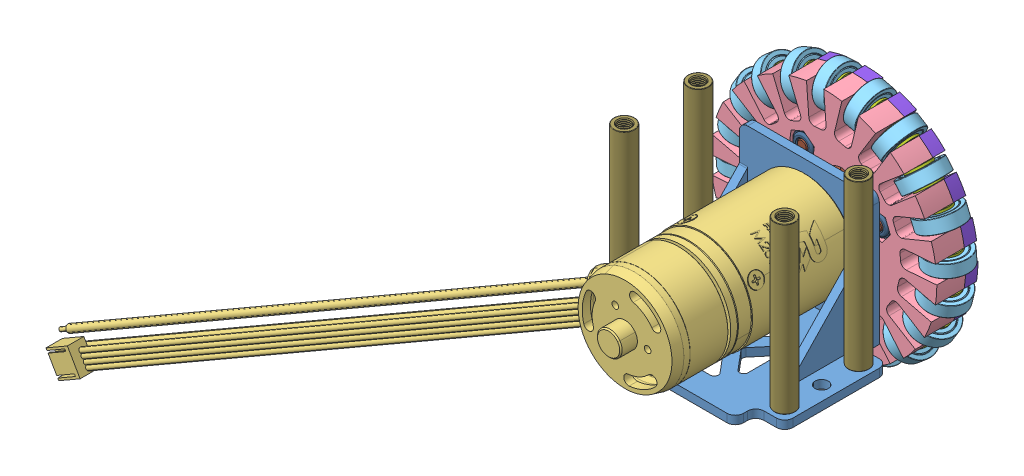
SolidWorks assembly RCSSL_gen2_OW_drive_unit, configuration Default. Lengths in mm.
Overall size (193.31 168.77 67.31).
123 component instances, 12 part files, 18 mates.
Components (placement in the parent):
- 1.5mm_aluminium_metal_plating_2006 motor mount-1: 1.5mm_aluminium_metal_plating_2006 motor mount [Default] at (10.7348 39.9667 23.6101) size (46 32 35)
- 3dp_AL_Gen2_Customised_AL_shaft_flange_connector_2006-1: 3dp_AL_Gen2_Customised_AL_shaft_flange_connector_2006 [Default] at (10.7348 39.9667 8.6101) x (0.866025 0.5 0) z (0 0 1) size (34 34 12.5)
- RoboMaster M2006 P36 motor 1-1: RoboMaster M2006 P36 motor 1 [默认] at (29.0021 49.1921 55.5053) x (0.258819 0.965926 0) z (0 0 1) size (137.53 138.78 64.81)
- ASM_RCssl_OW_Ver2-1: ASM_RCssl_OW_Ver2 [Default] at (25.0097 83.9716 -12.1645) x (-0.924615 -0.380903 0) z (0 0 1) size (59.33 59.33 15) (flexible)
  - 3dp_PETG_RCssl_OW_ver2_base-1: 3dp_PETG_RCssl_OW_ver2_base [Default] at (29.9603 35.2502 26.2746) size (54.84 54.84 7)
  - RCssl_OW_Ver2_roller_bearing_ASM-1: RCssl_OW_Ver2_roller_bearing_ASM [Default] at (24.4121 54.6156 21.3003) x (0 1 0) z (1 0 0) size (10 10 6)
    - BK_PU_68_3_10_3_bearing+roller-1: BK_PU_68_3_10_3_bearing+roller [Default] at (5.2981 6.4743 4.0482) size (10 10 3)
    - D3_H6_mid_axis-1: D3_H6_mid_axis [Default] at (5.2981 6.4743 2.5482) size (2.96 2.96 6)
    - m3_D6_H0.5_washer-1: m3_D6_H0.5_washer [Default] at (5.2981 6.4743 3.5482) x (0.872248 -0.489064 0) z (0 0 1) size (6 6 0.5)
    - m3_D6_H0.5_washer-2: m3_D6_H0.5_washer [Default] at (5.2981 6.4743 7.0482) size (6 6 0.5)
  - RCssl_OW_Ver2_roller_bearing_ASM-2: RCssl_OW_Ver2_roller_bearing_ASM [Default] at (30.6679 55.3823 21.3003) x (0.309017 0.951057 0) z (0.951057 -0.309017 0) size (10 10 6)
    - BK_PU_68_3_10_3_bearing+roller-1: BK_PU_68_3_10_3_bearing+roller [Default] at (5.2981 6.4743 4.0482) size (10 10 3)
    - D3_H6_mid_axis-1: D3_H6_mid_axis [Default] at (5.2981 6.4743 2.5482) size (2.96 2.96 6)
    - m3_D6_H0.5_washer-1: m3_D6_H0.5_washer [Default] at (5.2981 6.4743 3.5482) x (0.872248 -0.489064 0) z (0 0 1) size (6 6 0.5)
    - m3_D6_H0.5_washer-2: m3_D6_H0.5_washer [Default] at (5.2981 6.4743 7.0482) size (6 6 0.5)
  - RCssl_OW_Ver2_roller_bearing_ASM-3: RCssl_OW_Ver2_roller_bearing_ASM [Default] at (36.8544 54.1783 21.3003) x (0.587785 0.809017 0) z (0.809017 -0.587785 0) size (10 10 6)
    - BK_PU_68_3_10_3_bearing+roller-1: BK_PU_68_3_10_3_bearing+roller [Default] at (5.2981 6.4743 4.0482) size (10 10 3)
    - D3_H6_mid_axis-1: D3_H6_mid_axis [Default] at (5.2981 6.4743 2.5482) size (2.96 2.96 6)
    - m3_D6_H0.5_washer-1: m3_D6_H0.5_washer [Default] at (5.2981 6.4743 3.5482) x (0.872248 -0.489064 0) z (0 0 1) size (6 6 0.5)
    - m3_D6_H0.5_washer-2: m3_D6_H0.5_washer [Default] at (5.2981 6.4743 7.0482) size (6 6 0.5)
  - RCssl_OW_Ver2_roller_bearing_ASM-4: RCssl_OW_Ver2_roller_bearing_ASM [Default] at (42.3661 51.1215 21.3003) x (0.809017 0.587785 0) z (0.587785 -0.809017 0) size (10 10 6)
    - BK_PU_68_3_10_3_bearing+roller-1: BK_PU_68_3_10_3_bearing+roller [Default] at (5.2981 6.4743 4.0482) size (10 10 3)
    - D3_H6_mid_axis-1: D3_H6_mid_axis [Default] at (5.2981 6.4743 2.5482) size (2.96 2.96 6)
    - m3_D6_H0.5_washer-1: m3_D6_H0.5_washer [Default] at (5.2981 6.4743 3.5482) x (0.872248 -0.489064 0) z (0 0 1) size (6 6 0.5)
    - m3_D6_H0.5_washer-2: m3_D6_H0.5_washer [Default] at (5.2981 6.4743 7.0482) size (6 6 0.5)
  - RCssl_OW_Ver2_roller_bearing_ASM-5: RCssl_OW_Ver2_roller_bearing_ASM [Default] at (46.6634 46.5111 21.3003) x (0.951057 0.309017 0) z (0.309017 -0.951057 0) size (10 10 6)
    - BK_PU_68_3_10_3_bearing+roller-1: BK_PU_68_3_10_3_bearing+roller [Default] at (5.2981 6.4743 4.0482) size (10 10 3)
    - D3_H6_mid_axis-1: D3_H6_mid_axis [Default] at (5.2981 6.4743 2.5482) size (2.96 2.96 6)
    - m3_D6_H0.5_washer-1: m3_D6_H0.5_washer [Default] at (5.2981 6.4743 3.5482) x (0.872248 -0.489064 0) z (0 0 1) size (6 6 0.5)
    - m3_D6_H0.5_washer-2: m3_D6_H0.5_washer [Default] at (5.2981 6.4743 7.0482) size (6 6 0.5)
  - RCssl_OW_Ver2_roller_bearing_ASM-6: RCssl_OW_Ver2_roller_bearing_ASM [Default] at (49.3257 40.7985 21.3003) x (1 0 0) z (0 -1 0) size (10 10 6)
    - BK_PU_68_3_10_3_bearing+roller-1: BK_PU_68_3_10_3_bearing+roller [Default] at (5.2981 6.4743 4.0482) size (10 10 3)
    - D3_H6_mid_axis-1: D3_H6_mid_axis [Default] at (5.2981 6.4743 2.5482) size (2.96 2.96 6)
    - m3_D6_H0.5_washer-1: m3_D6_H0.5_washer [Default] at (5.2981 6.4743 3.5482) x (0.872248 -0.489064 0) z (0 0 1) size (6 6 0.5)
    - m3_D6_H0.5_washer-2: m3_D6_H0.5_washer [Default] at (5.2981 6.4743 7.0482) size (6 6 0.5)
  - RCssl_OW_Ver2_roller_bearing_ASM-7: RCssl_OW_Ver2_roller_bearing_ASM [Default] at (50.0924 34.5427 21.3003) x (0.951057 -0.309017 0) z (-0.309017 -0.951057 0) size (10 10 6)
    - BK_PU_68_3_10_3_bearing+roller-1: BK_PU_68_3_10_3_bearing+roller [Default] at (5.2981 6.4743 4.0482) size (10 10 3)
    - D3_H6_mid_axis-1: D3_H6_mid_axis [Default] at (5.2981 6.4743 2.5482) size (2.96 2.96 6)
    - m3_D6_H0.5_washer-1: m3_D6_H0.5_washer [Default] at (5.2981 6.4743 3.5482) x (0.872248 -0.489064 0) z (0 0 1) size (6 6 0.5)
    - m3_D6_H0.5_washer-2: m3_D6_H0.5_washer [Default] at (5.2981 6.4743 7.0482) size (6 6 0.5)
  - RCssl_OW_Ver2_roller_bearing_ASM-8: RCssl_OW_Ver2_roller_bearing_ASM [Default] at (48.8884 28.3562 21.3003) x (0.809017 -0.587785 0) z (-0.587785 -0.809017 0) size (10 10 6)
    - BK_PU_68_3_10_3_bearing+roller-1: BK_PU_68_3_10_3_bearing+roller [Default] at (5.2981 6.4743 4.0482) size (10 10 3)
    - D3_H6_mid_axis-1: D3_H6_mid_axis [Default] at (5.2981 6.4743 2.5482) size (2.96 2.96 6)
    - m3_D6_H0.5_washer-1: m3_D6_H0.5_washer [Default] at (5.2981 6.4743 3.5482) x (0.872248 -0.489064 0) z (0 0 1) size (6 6 0.5)
    - m3_D6_H0.5_washer-2: m3_D6_H0.5_washer [Default] at (5.2981 6.4743 7.0482) size (6 6 0.5)
  - RCssl_OW_Ver2_roller_bearing_ASM-9: RCssl_OW_Ver2_roller_bearing_ASM [Default] at (45.8316 22.8445 21.3003) x (0.587785 -0.809017 0) z (-0.809017 -0.587785 0) size (10 10 6)
    - BK_PU_68_3_10_3_bearing+roller-1: BK_PU_68_3_10_3_bearing+roller [Default] at (5.2981 6.4743 4.0482) size (10 10 3)
    - D3_H6_mid_axis-1: D3_H6_mid_axis [Default] at (5.2981 6.4743 2.5482) size (2.96 2.96 6)
    - m3_D6_H0.5_washer-1: m3_D6_H0.5_washer [Default] at (5.2981 6.4743 3.5482) x (0.872248 -0.489064 0) z (0 0 1) size (6 6 0.5)
    - m3_D6_H0.5_washer-2: m3_D6_H0.5_washer [Default] at (5.2981 6.4743 7.0482) size (6 6 0.5)
  - RCssl_OW_Ver2_roller_bearing_ASM-10: RCssl_OW_Ver2_roller_bearing_ASM [Default] at (41.2212 18.5472 21.3003) x (0.309017 -0.951057 0) z (-0.951057 -0.309017 0) size (10 10 6)
    - BK_PU_68_3_10_3_bearing+roller-1: BK_PU_68_3_10_3_bearing+roller [Default] at (5.2981 6.4743 4.0482) size (10 10 3)
    - D3_H6_mid_axis-1: D3_H6_mid_axis [Default] at (5.2981 6.4743 2.5482) size (2.96 2.96 6)
    - m3_D6_H0.5_washer-1: m3_D6_H0.5_washer [Default] at (5.2981 6.4743 3.5482) x (0.872248 -0.489064 0) z (0 0 1) size (6 6 0.5)
    - m3_D6_H0.5_washer-2: m3_D6_H0.5_washer [Default] at (5.2981 6.4743 7.0482) size (6 6 0.5)
  - RCssl_OW_Ver2_roller_bearing_ASM-11: RCssl_OW_Ver2_roller_bearing_ASM [Default] at (35.5086 15.8849 21.3003) x (0 -1 0) z (-1 0 0) size (10 10 6)
    - BK_PU_68_3_10_3_bearing+roller-1: BK_PU_68_3_10_3_bearing+roller [Default] at (5.2981 6.4743 4.0482) size (10 10 3)
    - D3_H6_mid_axis-1: D3_H6_mid_axis [Default] at (5.2981 6.4743 2.5482) size (2.96 2.96 6)
    - m3_D6_H0.5_washer-1: m3_D6_H0.5_washer [Default] at (5.2981 6.4743 3.5482) x (0.872248 -0.489064 0) z (0 0 1) size (6 6 0.5)
    - m3_D6_H0.5_washer-2: m3_D6_H0.5_washer [Default] at (5.2981 6.4743 7.0482) size (6 6 0.5)
  - RCssl_OW_Ver2_roller_bearing_ASM-12: RCssl_OW_Ver2_roller_bearing_ASM [Default] at (29.2528 15.1182 21.3003) x (-0.309017 -0.951057 0) z (-0.951057 0.309017 0) size (10 10 6)
    - BK_PU_68_3_10_3_bearing+roller-1: BK_PU_68_3_10_3_bearing+roller [Default] at (5.2981 6.4743 4.0482) size (10 10 3)
    - D3_H6_mid_axis-1: D3_H6_mid_axis [Default] at (5.2981 6.4743 2.5482) size (2.96 2.96 6)
    - m3_D6_H0.5_washer-1: m3_D6_H0.5_washer [Default] at (5.2981 6.4743 3.5482) x (0.872248 -0.489064 0) z (0 0 1) size (6 6 0.5)
    - m3_D6_H0.5_washer-2: m3_D6_H0.5_washer [Default] at (5.2981 6.4743 7.0482) size (6 6 0.5)
  - RCssl_OW_Ver2_roller_bearing_ASM-13: RCssl_OW_Ver2_roller_bearing_ASM [Default] at (23.0663 16.3222 21.3003) x (-0.587785 -0.809017 0) z (-0.809017 0.587785 0) size (10 10 6)
    - BK_PU_68_3_10_3_bearing+roller-1: BK_PU_68_3_10_3_bearing+roller [Default] at (5.2981 6.4743 4.0482) size (10 10 3)
    - D3_H6_mid_axis-1: D3_H6_mid_axis [Default] at (5.2981 6.4743 2.5482) size (2.96 2.96 6)
    - m3_D6_H0.5_washer-1: m3_D6_H0.5_washer [Default] at (5.2981 6.4743 3.5482) x (0.872248 -0.489064 0) z (0 0 1) size (6 6 0.5)
    - m3_D6_H0.5_washer-2: m3_D6_H0.5_washer [Default] at (5.2981 6.4743 7.0482) size (6 6 0.5)
  - RCssl_OW_Ver2_roller_bearing_ASM-14: RCssl_OW_Ver2_roller_bearing_ASM [Default] at (17.5546 19.379 21.3003) x (-0.809017 -0.587785 0) z (-0.587785 0.809017 0) size (10 10 6)
    - BK_PU_68_3_10_3_bearing+roller-1: BK_PU_68_3_10_3_bearing+roller [Default] at (5.2981 6.4743 4.0482) size (10 10 3)
    - D3_H6_mid_axis-1: D3_H6_mid_axis [Default] at (5.2981 6.4743 2.5482) size (2.96 2.96 6)
    - m3_D6_H0.5_washer-1: m3_D6_H0.5_washer [Default] at (5.2981 6.4743 3.5482) x (0.872248 -0.489064 0) z (0 0 1) size (6 6 0.5)
    - m3_D6_H0.5_washer-2: m3_D6_H0.5_washer [Default] at (5.2981 6.4743 7.0482) size (6 6 0.5)
  - RCssl_OW_Ver2_roller_bearing_ASM-15: RCssl_OW_Ver2_roller_bearing_ASM [Default] at (13.2573 23.9893 21.3003) x (-0.951057 -0.309017 0) z (-0.309017 0.951057 0) size (10 10 6)
    - BK_PU_68_3_10_3_bearing+roller-1: BK_PU_68_3_10_3_bearing+roller [Default] at (5.2981 6.4743 4.0482) size (10 10 3)
    - D3_H6_mid_axis-1: D3_H6_mid_axis [Default] at (5.2981 6.4743 2.5482) size (2.96 2.96 6)
    - m3_D6_H0.5_washer-1: m3_D6_H0.5_washer [Default] at (5.2981 6.4743 3.5482) x (0.872248 -0.489064 0) z (0 0 1) size (6 6 0.5)
    - m3_D6_H0.5_washer-2: m3_D6_H0.5_washer [Default] at (5.2981 6.4743 7.0482) size (6 6 0.5)
  - RCssl_OW_Ver2_roller_bearing_ASM-16: RCssl_OW_Ver2_roller_bearing_ASM [Default] at (10.595 29.702 21.3003) x (-1 0 0) z (0 1 0) size (10 10 6)
    - BK_PU_68_3_10_3_bearing+roller-1: BK_PU_68_3_10_3_bearing+roller [Default] at (5.2981 6.4743 4.0482) size (10 10 3)
    - D3_H6_mid_axis-1: D3_H6_mid_axis [Default] at (5.2981 6.4743 2.5482) size (2.96 2.96 6)
    - m3_D6_H0.5_washer-1: m3_D6_H0.5_washer [Default] at (5.2981 6.4743 3.5482) x (0.872248 -0.489064 0) z (0 0 1) size (6 6 0.5)
    - m3_D6_H0.5_washer-2: m3_D6_H0.5_washer [Default] at (5.2981 6.4743 7.0482) size (6 6 0.5)
  - RCssl_OW_Ver2_roller_bearing_ASM-17: RCssl_OW_Ver2_roller_bearing_ASM [Default] at (9.8283 35.9578 21.3003) x (-0.951057 0.309017 0) z (0.309017 0.951057 0) size (10 10 6)
    - BK_PU_68_3_10_3_bearing+roller-1: BK_PU_68_3_10_3_bearing+roller [Default] at (5.2981 6.4743 4.0482) size (10 10 3)
    - D3_H6_mid_axis-1: D3_H6_mid_axis [Default] at (5.2981 6.4743 2.5482) size (2.96 2.96 6)
    - m3_D6_H0.5_washer-1: m3_D6_H0.5_washer [Default] at (5.2981 6.4743 3.5482) x (0.872248 -0.489064 0) z (0 0 1) size (6 6 0.5)
    - m3_D6_H0.5_washer-2: m3_D6_H0.5_washer [Default] at (5.2981 6.4743 7.0482) size (6 6 0.5)
  - RCssl_OW_Ver2_roller_bearing_ASM-18: RCssl_OW_Ver2_roller_bearing_ASM [Default] at (11.0323 42.1443 21.3003) x (-0.809017 0.587785 0) z (0.587785 0.809017 0) size (10 10 6)
    - BK_PU_68_3_10_3_bearing+roller-1: BK_PU_68_3_10_3_bearing+roller [Default] at (5.2981 6.4743 4.0482) size (10 10 3)
    - D3_H6_mid_axis-1: D3_H6_mid_axis [Default] at (5.2981 6.4743 2.5482) size (2.96 2.96 6)
    - m3_D6_H0.5_washer-1: m3_D6_H0.5_washer [Default] at (5.2981 6.4743 3.5482) x (0.872248 -0.489064 0) z (0 0 1) size (6 6 0.5)
    - m3_D6_H0.5_washer-2: m3_D6_H0.5_washer [Default] at (5.2981 6.4743 7.0482) size (6 6 0.5)
  - RCssl_OW_Ver2_roller_bearing_ASM-19: RCssl_OW_Ver2_roller_bearing_ASM [Default] at (14.0891 47.656 21.3003) x (-0.587785 0.809017 0) z (0.809017 0.587785 0) size (10 10 6) (flexible)
    - BK_PU_68_3_10_3_bearing+roller-1: BK_PU_68_3_10_3_bearing+roller [Default] at (5.2981 6.4743 4.0482) size (10 10 3)
    - D3_H6_mid_axis-1: D3_H6_mid_axis [Default] at (5.2981 6.4743 2.5482) size (2.96 2.96 6)
    - m3_D6_H0.5_washer-1: m3_D6_H0.5_washer [Default] at (5.2981 6.4743 3.5482) x (0.872248 -0.489064 0) z (0 0 1) size (6 6 0.5)
    - m3_D6_H0.5_washer-2: m3_D6_H0.5_washer [Default] at (5.2981 6.4743 7.0482) size (6 6 0.5)
  - RCssl_OW_Ver2_roller_bearing_ASM-20: RCssl_OW_Ver2_roller_bearing_ASM [Default] at (18.6994 51.9533 21.3003) x (-0.309017 0.951057 0) z (0.951057 0.309017 0) size (10 10 6)
    - BK_PU_68_3_10_3_bearing+roller-1: BK_PU_68_3_10_3_bearing+roller [Default] at (5.2981 6.4743 4.0482) size (10 10 3)
    - D3_H6_mid_axis-1: D3_H6_mid_axis [Default] at (5.2981 6.4743 2.5482) size (2.96 2.96 6)
    - m3_D6_H0.5_washer-1: m3_D6_H0.5_washer [Default] at (5.2981 6.4743 3.5482) x (0.872248 -0.489064 0) z (0 0 1) size (6 6 0.5)
    - m3_D6_H0.5_washer-2: m3_D6_H0.5_washer [Default] at (5.2981 6.4743 7.0482) size (6 6 0.5)
  - CF3mm_OW_gen2_output_plane-1: CF3mm_OW_gen2_output_plane [Default] at (29.9603 35.2502 44.7746) size (54.84 54.84 3)
  - 3dp_PETG_RCssl_OW_front_lock-1: 3dp_PETG_RCssl_OW_front_lock [Default] at (29.9603 35.2502 21.2746) x (1 0 0) z (0 0 -1) size (21.15 21.15 4.13)
  - nut_din_985-m3x0_5-8-1: nut_din_985-m3x0_5-8 [Default] at (29.9603 21.2502 29.2746) x (-1 0 0) z (0 0 -1) size (6.2 5.5 4)
  - nut_din_985-m3x0_5-8-2: nut_din_985-m3x0_5-8 [Default] at (15.9603 35.2502 29.2746) x (0 1 0) z (0 0 -1) size (6.2 5.5 4)
  - nut_din_985-m3x0_5-8-3: nut_din_985-m3x0_5-8 [Default] at (29.9603 49.2502 29.2746) x (1 0 0) z (0 0 -1) size (6.2 5.5 4)
  - nut_din_985-m3x0_5-8-4: nut_din_985-m3x0_5-8 [Default] at (43.9603 35.2502 29.2746) x (0 -1 0) z (0 0 -1) size (6.2 5.5 4)
  - M3_304__full_teeth__screw_10mm-1: M3_304__full_teeth__screw_10mm [Default] at (29.992 49.2503 23.2746) x (-0.002323 0.999997 0) z (0 0 -1) size (5.3 5.3 13)
  - M3_304__full_teeth__screw_10mm-2: M3_304__full_teeth__screw_10mm [Default] at (43.9604 35.2186 23.2746) x (0.999997 0.002323 0) z (0 0 -1) size (5.3 5.3 13)
  - M3_304__full_teeth__screw_10mm-3: M3_304__full_teeth__screw_10mm [Default] at (29.9287 21.2502 23.2746) x (0.002323 -0.999997 0) z (0 0 -1) size (5.3 5.3 13)
  - M3_304__full_teeth__screw_10mm-4: M3_304__full_teeth__screw_10mm [Default] at (15.9603 35.2819 23.2746) x (-0.999997 -0.002323 0) z (0 0 -1) size (5.3 5.3 13)
  - M3_304__full_teeth__screw_10mm-5: M3_304__full_teeth__screw_10mm [Default] at (37.0442 42.2923 21.2746) x (0.914728 0.40407 0) z (0 0 -1) size (5.3 5.3 13)
  - M3_304__full_teeth__screw_10mm-6: M3_304__full_teeth__screw_10mm [Default] at (37.0024 28.1664 21.2746) x (0.40407 -0.914728 0) z (0 0 -1) size (5.3 5.3 13)
  - M3_304__full_teeth__screw_10mm-7: M3_304__full_teeth__screw_10mm [Default] at (22.8765 28.2081 21.2746) x (-0.914728 -0.40407 0) z (0 0 -1) size (5.3 5.3 13)
  - M3_304__full_teeth__screw_10mm-8: M3_304__full_teeth__screw_10mm [Default] at (22.9182 42.3341 21.2746) x (-0.40407 0.914728 0) z (0 0 -1) size (5.3 5.3 13)
- AL_pillar_M3_D6_H40_Threaded-2: AL_pillar_M3_D6_H40_Threaded [H30] at (-8.7652 24.9667 50.1101) size (5 40 5)
- AL_pillar_M3_D6_H40_Threaded-3: AL_pillar_M3_D6_H40_Threaded [H30] at (30.2348 24.9667 50.1101) size (5 40 5)
- AL_pillar_M3_D6_H40_Threaded-4: AL_pillar_M3_D6_H40_Threaded [Default] at (30.2348 24.9667 32.1101) x (0.546545 0 0.83743) z (-0.83743 0 0.546545) size (5 40 5)
- AL_pillar_M3_D6_H40_Threaded-5: AL_pillar_M3_D6_H40_Threaded [Default] at (-8.7652 24.9667 32.1101) x (0.546545 0 0.83743) z (-0.83743 0 0.546545) size (5 40 5)
Mates (geometry in assembly coordinates):
- Concentric1: concentric aligned: cylinder of 1.5mm_aluminium_metal_plating_2006 motor mount-1 through (10.7348 39.9667 25.6101) axis (0 0 -1) radius 7.25; cylinder of RoboMaster M2006 P36 motor 1-1 through (10.7348 39.9667 8.6101) axis (0 0 -1) radius 3
- Coincident1: coincident anti-aligned: plane of 1.5mm_aluminium_metal_plating_2006 motor mount-1 through (10.7348 39.9667 25.6101) normal (0 0 1); plane of RoboMaster M2006 P36 motor 1-1 through (21.3003 46.0667 25.6101) normal (0 0 -1)
- Concentric3: concentric aligned: cylinder of 3dp_AL_Gen2_Customised_AL_shaft_flange_connector_2006-1 through (10.7348 39.9667 20.1101) axis (0 0 -1) radius 3.075; cylinder of RoboMaster M2006 P36 motor 1-1 through (10.7348 39.9667 8.6101) axis (0 0 -1) radius 3
- Concentric6: concentric aligned: cylinder of 3dp_AL_Gen2_Customised_AL_shaft_flange_connector_2006-1 through (-13.9469 25.7167 17.6101) axis (0.866025 0.5 0) radius 1.55; cylinder of RoboMaster M2006 P36 motor 1-1 through (12.8999 41.2167 17.6101) axis (0.866025 0.5 0) radius 1.5
- Concentric7: concentric anti-aligned: cylinder of 1.5mm_aluminium_metal_plating_2006 motor mount-1 through (-8.7652 -2.9948 32.1101) axis (0 1 0) radius 1.6; cylinder of AL_pillar_M3_D6_H40_Threaded-1 through (-8.7652 64.9667 32.1101) axis (0 -1 0) radius 2.5
- Concentric8: concentric anti-aligned: cylinder of 1.5mm_aluminium_metal_plating_2006 motor mount-1 through (-8.7652 -2.9948 50.1101) axis (0 1 0) radius 1.6; cylinder of AL_pillar_M3_D6_H40_Threaded-2 through (-8.7652 64.9667 50.1101) axis (0 -1 0) radius 2.5
- Concentric9: concentric anti-aligned: cylinder of 1.5mm_aluminium_metal_plating_2006 motor mount-1 through (30.2348 -2.9948 50.1101) axis (0 1 0) radius 1.6; cylinder of AL_pillar_M3_D6_H40_Threaded-3 through (30.2348 64.9667 50.1101) axis (0 -1 0) radius 2.5
- Concentric10: concentric anti-aligned: cylinder of 1.5mm_aluminium_metal_plating_2006 motor mount-1 through (30.2348 -2.9948 32.1101) axis (0 1 0) radius 1.6; cylinder of AL_pillar_M3_D6_H40_Threaded-4 through (30.2348 64.9667 32.1101) axis (0 -1 0) radius 2.5
- Coincident3: coincident anti-aligned: plane of 1.5mm_aluminium_metal_plating_2006 motor mount-1 through (10.7348 24.9667 58.6101) normal (0 1 0); plane of AL_pillar_M3_D6_H40_Threaded-3 through (30.2348 24.9667 50.1101) normal (0 -1 0)
- Coincident4: coincident anti-aligned: plane of 1.5mm_aluminium_metal_plating_2006 motor mount-1 through (10.7348 24.9667 58.6101) normal (0 1 0); plane of AL_pillar_M3_D6_H40_Threaded-4 through (30.2348 24.9667 32.1101) normal (0 -1 0)
- Coincident5: coincident anti-aligned: plane of 1.5mm_aluminium_metal_plating_2006 motor mount-1 through (10.7348 24.9667 58.6101) normal (0 1 0); plane of AL_pillar_M3_D6_H40_Threaded-2 through (-8.7652 24.9667 50.1101) normal (0 -1 0)
- Coincident6: coincident anti-aligned: plane of 1.5mm_aluminium_metal_plating_2006 motor mount-1 through (10.7348 24.9667 58.6101) normal (0 1 0); plane of AL_pillar_M3_D6_H40_Threaded-1 through (-8.7652 24.9667 32.1101) normal (0 -1 0)
- Concentric12: concentric aligned: cylinder of RoboMaster M2006 P36 motor 1-1 through (10.7348 39.9667 8.6101) axis (0 0 -1) radius 3; cylinder of ASM_RCssl_OW_Ver2-1/CF3mm_OW_gen2_output_plane-1 through (10.7348 39.9667 33.1101) axis (0 0 -1) radius 3.05
- Concentric13: concentric aligned: cylinder of 1.5mm_aluminium_metal_plating_2006 motor mount-1 through (2.5075 44.7167 33.6101) axis (0 0 -1) radius 1.5; cylinder of RoboMaster M2006 P36 motor 1-1 through (2.5075 44.7167 25.6101) axis (0 0 -1) radius 1.25
- Concentric14: concentric anti-aligned: cylinder of 1.5mm_aluminium_metal_plating_2006 motor mount-1 through (30.2348 -2.9948 32.1101) axis (0 1 0) radius 1.6; cylinder of AL_pillar_M3_D6_H40_Threaded-4 through (30.2348 64.9667 32.1101) axis (0 -1 0) radius 2.5
- Concentric15: concentric anti-aligned: cylinder of 1.5mm_aluminium_metal_plating_2006 motor mount-1 through (-8.7652 -2.9948 32.1101) axis (0 1 0) radius 1.6; cylinder of AL_pillar_M3_D6_H40_Threaded-5 through (-8.7652 64.9667 32.1101) axis (0 -1 0) radius 2.5
- Coincident7: coincident anti-aligned: plane of 1.5mm_aluminium_metal_plating_2006 motor mount-1 through (10.7348 24.9667 58.6101) normal (0 1 0); plane of AL_pillar_M3_D6_H40_Threaded-5 through (-8.7652 24.9667 32.1101) normal (0 -1 0)
- Coincident8: coincident anti-aligned: plane of 3dp_AL_Gen2_Customised_AL_shaft_flange_connector_2006-1 through (-3.8905 43.2985 14.1101) normal (0 0 -1); plane of ASM_RCssl_OW_Ver2-1/CF3mm_OW_gen2_output_plane-1 through (13.0604 20.123 14.1101) normal (0 0 1)
